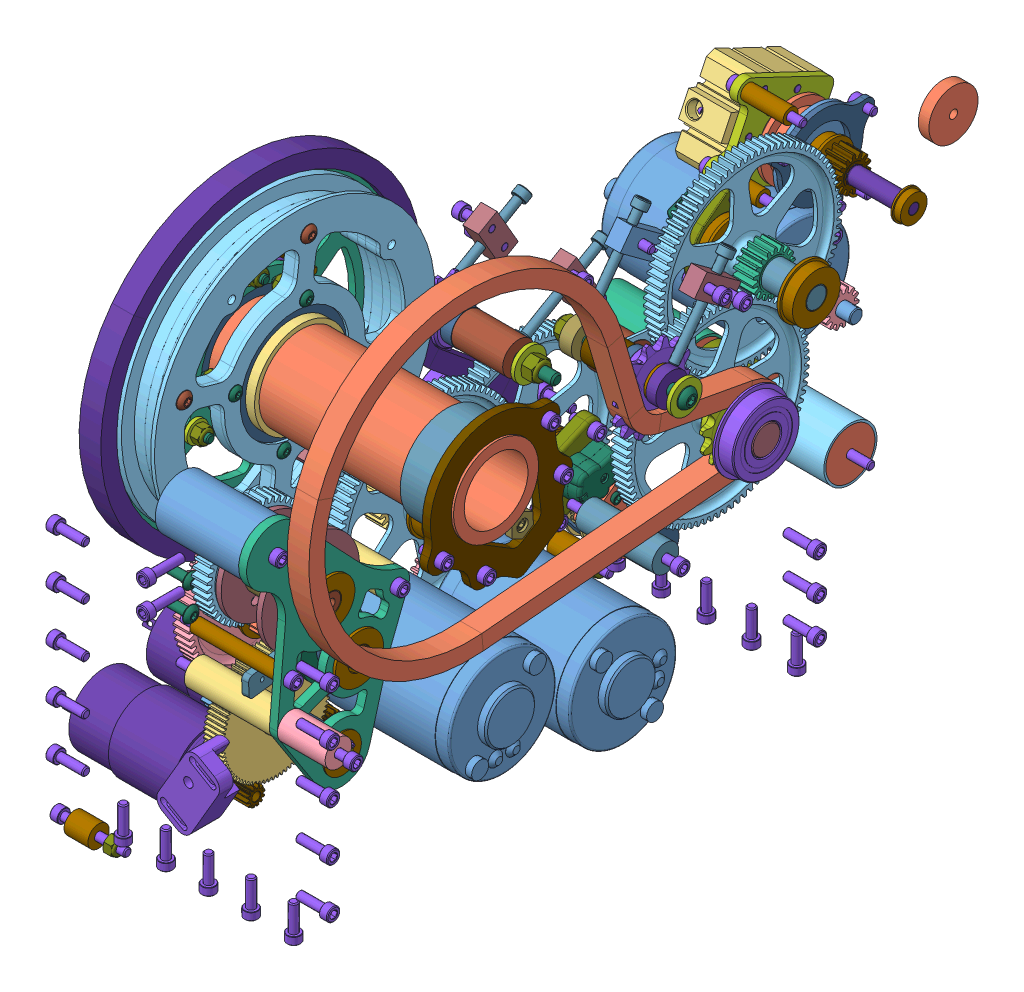
SolidWorks assembly 971-18-A-2900_Arm Gearbox, configuration Default. Lengths in mm.
Overall size (180.27 346.15 436.67).
321 component instances, 101 part files, 306 mates.
Components (placement in the parent):
- 971-18-P-0057_Arm Gearbox Plates-1: 971-18-P-0057_Arm Gearbox Plates [Not Hanger Plates] at origin size (158.75 274.35 412.07) (hidden)
- MiniCIM-1: MiniCIM [Default] at (101.9302 -45.1539 -242.57) x (-1 0 0) z (0 -0.56592 -0.82446) size (125.82 64.26 64.26)
- 971-18-P-0063_Proximal Joint Chain-1: 971-18-P-0063_Proximal Joint Chain [Default] at (142.3112 0 0) x (-1 0 0) z (0 0.942809 -0.333333) size (12.95 293.93 191.44)
- MiniCIM-2: MiniCIM [Default] at (68.2625 -128.7803 -15.3525) x (1 0 0) z (0 0.733761 -0.679407) size (125.82 64.26 64.26)
- 28T-1_2-Hex-Steel_217-5468-1: 28T-1_2-Hex-Steel_217-5468 [Default] at (42.9633 -91.1077 -64.9795) x (0 0.556138 -0.83109) z (-1 0 0) size (38.56 38.56 12.6)
- 14T-CIM_217-3414-1: 14T-CIM_217-3414 [default] at (44.9112 -128.7803 -15.3525) x (0 -0.350281 -0.936645) z (-1 0 0) size (20.32 20.6 19.05)
- 971-18-P-0186_84T Gear With Access Hole-1: 971-18-P-0186_84T Gear With Access Hole [Default] at (42.9879 -103.4997 -135.089) x (0 -0.686618 -0.727018) z (1 0 0) size (109.49 109.49 12.65)
- 971-18-P-0186_84T Gear With Access Hole-2: 971-18-P-0186_84T Gear With Access Hole [Default] at (55.5879 -91.1077 -64.9795) x (0 -0.395137 -0.918622) z (-1 0 0) size (109.49 109.49 12.65)
- 971-18-P-0186_84T Gear With Access Hole-3: 971-18-P-0186_84T Gear With Access Hole [Default] at (114.8094 -2.1568 -197.4778) x (0 0.448525 0.89377) z (-1 0 0) size (109.49 109.49 12.65)
- 971-18-P-0186_84T Gear With Access Hole-4: 971-18-P-0186_84T Gear With Access Hole [Default] at (127.4586 -58.42 -165.2367) x (0 0.119081 -0.992885) z (-1 0 0) size (109.49 109.49 12.65)
- 18T-1_2-Hex-Steel_217-5460-2: 18T-1_2-Hex-Steel_217-5460 [Default] at (127.4339 -2.1568 -197.4778) x (0 -0.996212 -0.086957) z (1 0 0) size (25.65 25.85 12.6)
- 12T_Hex_217-2662-2: 12T_Hex_217-2662 [Default] at (18.0263 -103.4997 -135.089) x (0 -0.568149 -0.822926) z (1 0 0) size (40.29 40.29 10.67)
- 6661K350_17mm ID 40mm OD BALL BEARING-2: 6661K350_17mm ID 40mm OD BALL BEARING [6661K35] at (3.53 -103.4997 -135.089) x (0 0 1) z (1 0 0) size (44.6 44.6 12)
- MiniCIM-3: MiniCIM [Default] at (68.2625 -149.225 -87.4394) x (1 0 0) z (0 0.801756 0.597652) size (125.82 64.26 64.26)
- 14T-CIM_217-3414-2: 14T-CIM_217-3414 [default] at (44.9112 -149.225 -87.4394) x (0 0.658796 0.752321) z (-1 0 0) size (20.32 20.6 19.05)
- 14T-CIM_217-3414-3: 14T-CIM_217-3414 [default] at (119.605 -45.1539 -242.57) x (0 0.994685 -0.102967) z (-1 0 0) size (20.32 20.6 19.05)
- Bearings-1: Bearings [0.5 ID, 1.125 OD, 0.313 Width, Flanged, FR8-ZZ] at (65.8876 -103.4997 -135.089) x (0 -0.204169 -0.978936) z (1 0 0) size (31.12 31.12 7.95)
- Bearings-2: Bearings [0.5 ID, 1.125 OD, 0.313 Width, Flanged, FR8-ZZ] at (3.9624 -91.1077 -64.9795) x (0 -0.438567 -0.898699) z (-1 0 0) size (31.12 31.12 7.95)
- Bearings-4: Bearings [0.5 ID, 1.125 OD, 0.313 Width, Flanged, FR8-ZZ] at (154.7876 -2.1568 -197.4778) x (0 -0.31213 0.950039) z (1 0 0) size (31.12 31.12 7.95)
- Bearings-5: Bearings [0.5 ID, 1.125 OD, 0.313 Width, Flanged, FR8-ZZ] at (104.3051 -2.1568 -197.4778) x (0 0.974827 0.222965) z (-1 0 0) size (31.12 31.12 7.95)
- Bearings-6: Bearings [0.5 ID, 1.125 OD, 0.313 Width, Flanged, FR8-ZZ] at (65.8876 -91.1077 -64.9795) x (0 0.620593 0.784133) z (1 0 0) size (31.12 31.12 7.95)
- 12T_Hex_217-2662-5: 12T_Hex_217-2662 [Default] at (142.3112 -58.42 -165.2367) x (0 -0.053723 0.998556) z (-1 0 0) size (40.29 40.29 10.67)
- 6661K350_17mm ID 40mm OD BALL BEARING-3: 6661K350_17mm ID 40mm OD BALL BEARING [6661K35] at (155.22 -58.42 -165.2367) x (0 -0.924225 -0.381849) z (-1 0 0) size (44.6 44.6 12)
- 3549S-1BA-102B-ND 10 turn potentiometer-1: 3549S-1BA-102B-ND 10 turn potentiometer [Default] at (93.141 -149.8585 -169.7731) x (0 -0.445388 -0.895338) z (-1 0 0) size (22.48 22.48 39.06)
- 3547S-1AA-102A-ND 3 Turn Potentiometer Bourns-2: 3547S-1AA-102A-ND 3 Turn Potentiometer Bourns [Default] at (64.1081 -58.42 -165.2367) x (0 0.520541 -0.853837) z (1 0 0) size (22.48 22.48 39.06)
- Bearings-9: Bearings [0.5 ID, 1.125 OD, 0.313 Width, Flanged, FR8-ZZ] at (104.3051 -58.42 -165.2367) x (0 -0.997236 -0.074294) z (-1 0 0) size (31.12 31.12 7.95)
- SHCS-1: SHCS [6.5, #10-32] at (82.55 45.4322 -285.7008) x (1 0 0) z (0 -0.658646 -0.752453) size (170.15 7.92 7.92) (hidden)
- SRK Mag Encoder Magnet-1: SRK Mag Encoder Magnet [Default] at (63.0047 -103.4997 -135.089) x (0 0.994372 0.105943) z (0 0.105943 -0.994372) size (6.35 12.7 6.35)
- SRK Mag Encoder Magnet-2: SRK Mag Encoder Magnet [Default] at (107.2515 -2.1568 -197.4778) x (0 -0.949695 0.313176) z (0 -0.313176 -0.949695) size (6.35 12.7 6.35)
- 971-18-P-0104_Arm Gearbox Proximal Arm Output Shaft-1: 971-18-P-0104_Arm Gearbox Proximal Arm Output Shaft [Default] at (161.22 -58.42 -165.2367) x (0 0.817505 0.575921) z (1 0 0) size (19.05 19.05 69.68)
- 971-18-P-0105_Arm Gearbox Proximal Arm First Stage Shaft -1: 971-18-P-0105_Arm Gearbox Proximal Arm First Stage Shaft  [Default] at (133.7437 -2.1568 -197.4778) x (0 0 -1) z (1 0 0) size (15.88 15.88 58.37)
- 971-18-P-0106_Arm Gearbox Distal Arm First Stage Shaft-1: 971-18-P-0106_Arm Gearbox Distal Arm First Stage Shaft [Default] at (69.8627 -91.1077 -64.9795) x (0 0 -1) z (1 0 0) size (15.88 15.88 69.88)
- 971-18-P-0107_Arm Gearbox Distal Arm Output Shaft-1: 971-18-P-0107_Arm Gearbox Distal Arm Output Shaft [Default] at (69.8627 -103.4997 -135.089) x (0 0.391562 -0.920152) z (1 0 0) size (19.05 19.05 72.33)
- 971-18-P-0070_Distal Joint Chain-1: 971-18-P-0070_Distal Joint Chain [Default] at (18.0263 0 0) x (-1 0 0) z (0 0.793801 -0.608178) size (12.95 288.85 191.44)
- 971-18-P-0101_Tensioner Strap-1: 971-18-P-0101_Tensioner Strap [Default] x (-1 0 0) z (0 0.537919 -0.842996) size (4.76 92.32 90.96)
- 971-18-P-0101_Tensioner Strap-2: 971-18-P-0101_Tensioner Strap [Default] at (163.5125 0 0) x (-1 0 0) z (0 0.537919 -0.842996) size (4.76 92.32 90.96)
- potentiometer belt-1: potentiometer belt [Default] at (51.6937 -103.4997 -135.089) x (1 0 0) z (0 0.800703 0.599061) size (6.35 27.13 83.74)
- 971-18-P-0112_Arm Gearbox Distal Potentiometer Mount-1: 971-18-P-0112_Arm Gearbox Distal Potentiometer Mount [Default] at (74.695 -149.8585 -169.7731) x (-1 0 0) z (0 0.599061 -0.800703) size (8.89 42.86 25.08)
- A-6z16-036df2508_36t plastic pulley-1: A-6z16-036df2508_36t plastic pulley [Default] at (54.8687 -149.8585 -169.7731) x (0 -0.600937 0.799296) z (1 0 0) size (27.69 27.69 17.46)
- 971-18-P-0254_40T plastic pulley hex-1: 971-18-P-0254_40T plastic pulley hex [Default] at (54.8687 -103.4997 -135.089) x (0 -0.910247 0.414066) z (-1 0 0) size (30.23 30.23 11.11)
- 971-18-P-0116_Arm Proximal Side Spacer-1: 971-18-P-0116_Arm Proximal Side Spacer [Default] at (129.54 -99.4146 -224.1283) x (1 0 0) z (0 -0.998204 -0.059903) size (45.72 31.75 31.75)
- 971-18-P-0116_Arm Proximal Side Spacer-2: 971-18-P-0116_Arm Proximal Side Spacer [Default] at (129.54 45.4322 -285.7008) x (1 0 0) z (0 -0.135571 0.990768) size (45.72 31.75 31.75) (hidden)
- 971-18-P-0115_Arm Distal Side Spacer-1: 971-18-P-0115_Arm Distal Side Spacer [Default] at (34.925 -99.4146 -224.1283) x (1 0 0) z (0 -0.874507 -0.485014) size (57.15 31.75 31.75)
- 971-18-P-0115_Arm Distal Side Spacer-2: 971-18-P-0115_Arm Distal Side Spacer [Default] at (34.925 -166.289 -43.6572) x (1 0 0) z (0 0.434751 -0.900551) size (57.15 31.75 31.75)
- 971-18-P-0118_Arm Distal Side Double Spacer-1: 971-18-P-0118_Arm Distal Side Double Spacer [Default] at (54.1401 45.4322 -285.7008) x (1 0 0) z (0 -0.790861 -0.611996) size (95.58 31.75 31.75) (hidden)
- 971-18-A-4500_Arm Tensioner Idler-1: 971-18-A-4500_Arm Tensioner Idler [Default] at (136.9581 -12.6592 -117.4327) x (0 0.639462 0.768823) z (-1 0 0) size (46.24 46.24 19.05)
  - 8491A293_0_5 OD PRESS-FIT DRILL BUSHING-1: 8491A293_0_5 OD PRESS-FIT DRILL BUSHING [8491A293] at origin size (12.7 12.7 19.05)
  - 971-18-P-0119_Arm Tensioner Idler-1: 971-18-P-0119_Arm Tensioner Idler [Default] at (0 0 -5.353) x (0.987019 -0.160606 0) z (0 0 1) size (40.29 40.29 10.67)
  - 5905K230_0_5ID STEEL NEEDLE-ROLLER BEARING-1: 5905K230_0_5ID STEEL NEEDLE-ROLLER BEARING [5905K23] at (0 0 -3.175) size (17.46 17.46 12.7)
  - VexPro_Hex Spacers-2: VexPro_Hex Spacers [1_2 Hex, 0.25] at (0 0 6.35) x (0.957977 0.286844 0) z (0 0 1) size (19.51 19.51 6.35)
- 971-18-A-4500_Arm Tensioner Idler-2: 971-18-A-4500_Arm Tensioner Idler [Default] at (23.3793 -39.637 -114.8895) x (0 -0.847075 -0.531473) z (1 0 0) size (46.24 46.24 19.05)
  - 8491A293_0_5 OD PRESS-FIT DRILL BUSHING-1: 8491A293_0_5 OD PRESS-FIT DRILL BUSHING [8491A293] at origin size (12.7 12.7 19.05)
  - 971-18-P-0119_Arm Tensioner Idler-1: 971-18-P-0119_Arm Tensioner Idler [Default] at (0 0 -5.353) x (0.987019 -0.160606 0) z (0 0 1) size (40.29 40.29 10.67)
  - 5905K230_0_5ID STEEL NEEDLE-ROLLER BEARING-1: 5905K230_0_5ID STEEL NEEDLE-ROLLER BEARING [5905K23] at (0 0 -3.175) size (17.46 17.46 12.7)
  - VexPro_Hex Spacers-2: VexPro_Hex Spacers [1_2 Hex, 0.25] at (0 0 6.35) x (0.957977 0.286844 0) z (0 0 1) size (19.51 19.51 6.35)
- 971-18-P-0122_Distal Tensioner Long Spacer-1: 971-18-P-0122_Distal Tensioner Long Spacer [Default] at (48.1951 -39.637 -114.8895) x (0 0 1) z (-1 0 0) size (19.05 19.05 30.58)
- 971-18-P-0123_Distal Tensioner Short Spacer-1: 971-18-P-0123_Distal Tensioner Short Spacer [Default] at (10.1078 -39.637 -114.8895) x (0 0.086251 0.996273) z (-1 0 0) size (19.05 19.05 7.49)
- 971-18-P-0124_Sketchy Chain Tensioner-1: 971-18-P-0124_Sketchy Chain Tensioner [Default] at (11.1125 -19.1237 -150.4225) x (1 0 0) z (0 0.866025 0.5) size (9.53 12.7 25.4)
- 90044A120_2-in Full Thread BLACK-OXIDE ALLOY STEEL SOCKET HEAD CAP SCREW-1: 90044A120_2-in Full Thread BLACK-OXIDE ALLOY STEEL SOCKET HEAD CAP SCREW [90044A120] at (11.1125 -22.1758 -145.1362) x (0 -0.5 0.866025) z (-0.011915 0.865964 0.499965) size (55.85 7.92 7.92)
- 971-18-P-0124_Sketchy Chain Tensioner-2: 971-18-P-0124_Sketchy Chain Tensioner [Default] at (58.7375 -19.1237 -150.4225) x (1 0 0) z (0 0.866025 0.5) size (9.53 12.7 25.4)
- 90044A120_2-in Full Thread BLACK-OXIDE ALLOY STEEL SOCKET HEAD CAP SCREW-2: 90044A120_2-in Full Thread BLACK-OXIDE ALLOY STEEL SOCKET HEAD CAP SCREW [90044A120] at (58.7375 -22.1758 -145.1362) x (0 -0.5 0.866025) z (-0.011915 0.865964 0.499965) size (55.85 7.92 7.92)
- BHCS-1: BHCS [3.5, .25-20] at (-5.6388 -39.637 -114.8895) x (0 0 1) z (-1 0 0) size (11.1 11.1 92.48)
- Nylon-Insert Locknut-1: Nylon-Insert Locknut [.25-20  Nylon-Insert Locknut] at (70.5485 -39.637 -114.8895) x (0 -0.87684 0.480783) z (0 0.480783 0.87684) size (11.11 7.94 12.83)
- 971-18-P-0248_Proximal Tensioner Short Spacer-2: 971-18-P-0248_Proximal Tensioner Short Spacer [Default] at (149.4359 -12.6592 -117.4327) x (0 -0.700571 0.713583) z (-1 0 0) size (19.05 19.05 5.91)
- 971-18-P-0124_Sketchy Chain Tensioner-3: 971-18-P-0124_Sketchy Chain Tensioner [Default] at (147.6375 24.7667 -144.9822) x (1 0 0) z (0 0.592784 0.805361) size (9.53 12.7 25.4)
- 90044A120_2-in Full Thread BLACK-OXIDE ALLOY STEEL SOCKET HEAD CAP SCREW-3: 90044A120_2-in Full Thread BLACK-OXIDE ALLOY STEEL SOCKET HEAD CAP SCREW [90044A120] at (147.6375 15.467 -138.1372) x (0 -0.805361 0.592784) z (-0.011915 0.592742 0.805304) size (55.85 7.92 7.92)
- 971-18-P-0125_Proximal Tensioner Long Spacer-1: 971-18-P-0125_Proximal Tensioner Long Spacer [Default] at (117.07 -12.6592 -117.4327) x (0 0 -1) z (1 0 0) size (17.78 17.78 20.73)
- 90044A120_2-in Full Thread BLACK-OXIDE ALLOY STEEL SOCKET HEAD CAP SCREW-4: 90044A120_2-in Full Thread BLACK-OXIDE ALLOY STEEL SOCKET HEAD CAP SCREW [90044A120] at (97.1677 14.9556 -137.7608) x (0 -0.805361 0.592784) z (0.19068 0.581908 0.790585) size (55.85 7.92 7.92)
- BHCS-2: BHCS [3, .25-20] at (164.3888 -12.6592 -117.4327) x (0 -0.924225 -0.381849) z (1 0 0) size (11.1 11.1 79.78)
- Nylon-Insert Locknut-2: Nylon-Insert Locknut [.25-20  Nylon-Insert Locknut] at (94.4372 -12.6592 -117.4327) x (0 -0.381849 0.924225) z (0 -0.924225 -0.381849) size (11.11 7.94 12.83)
- 971-18-P-0123_Distal Tensioner Short Spacer-3: 971-18-P-0123_Distal Tensioner Short Spacer [Default] at (98.1837 -12.6592 -117.4327) x (0 -0.700571 0.713583) z (-1 0 0) size (19.05 19.05 7.49)
- 971-18-P-0264_Swoopy thing 2-1: 971-18-P-0264_Swoopy thing 2 [Default] at (97.1677 24.7667 -144.9822) x (1 0 0) z (0 -0.592784 -0.805361) size (9.53 12.7 29.21)
- 971-18-P-0119_Arm Tensioner Idler-1: 971-18-P-0119_Arm Tensioner Idler [Default] at (142.3112 -18.7027 -112.9867) x (0 0.507683 0.861544) z (-1 0 0) size (40.29 40.29 10.67)
- 971-18-A-4800_Arm Base Axle-1: 971-18-A-4800_Arm Base Axle [Default] at (79.375 0 0) x (0 0.839057 0.544043) z (1 0 0) size (228.13 188.75 173.98)
  - 971-18-P-0098_Proximal Shoulder Joint Tube Shaft-1: 971-18-P-0098_Proximal Shoulder Joint Tube Shaft [Default] at origin size (50.8 50.8 173.98)
  - 971-18-P-0109_Arm to Capstan Spacer-1: 971-18-P-0109_Arm to Capstan Spacer [Default] at (0 0 -33.6475) size (55.56 55.56 5.38)
  - 971-18-P-0110_Capstan to Gearbox Spacer-1: 971-18-P-0110_Capstan to Gearbox Spacer [Default] at (0 0 -70.6322) x (0.975154 0.22153 0) z (0 0 1) size (55.56 55.56 4.72)
  - 971-18-A-2700_Distal Joint Base Sprocket-1: 971-18-A-2700_Distal Joint Base Sprocket [Default] at (0 0 -45.7212) x (0 0 -1) z (-0.006536 0.999979 0) size (39.06 226.91 187.27)
    - 971-18-P-0065_Distal Joint Capstan-1: 971-18-P-0065_Distal Joint Capstan [Default] at origin size (24.51 167.64 167.64)
    - 971-18-P-0069_Distal Base Sprocket, 60T #35-1: 971-18-P-0069_Distal Base Sprocket, 60T #35 [Default] at (15.64 0 0) x (0 0 1) z (-1 0 0) size (187.27 187.27 4.29)
    - Mock Allen Key-1: Mock Allen Key [Default] at (0 33.0633 -17.145) x (0.575263 0.315216 -0.754792) z (0.20677 -0.948834 -0.238663) size (4.57 4.57 127) (hidden)
    - 91525A318_No8 Oversized Washer-1: 91525A318_No8 Oversized Washer [91525A318] at (-2.3813 -26.2838 -25.4) x (1 0 0) z (0 0.858193 0.513327) size (2.03 12.7 12.7)
    - Nylon-Insert Locknut-1: Nylon-Insert Locknut [#8-32  Nylon-Insert Locknut] at (-0.3493 -26.2838 -25.4) x (0 -0.163443 -0.986553) z (0 -0.986553 0.163443) size (8.73 5.95 10.08)
    - 971-18-P-0067_Distal Sprocket Bearing Reinforcement-1: 971-18-P-0067_Distal Sprocket Bearing Reinforcement [Default] at (17.7863 0 0) x (1 0 0) z (0 0.5 0.866025) size (4.76 97.7 86.31)
    - BHCS-4: BHCS [0.75, #10-32] at (25.1143 -36.8061 -21.25) x (0 -0.437304 -0.899314) z (1 0 0) size (9.17 9.17 21.8)
    - Dowel Pins-1: Dowel Pins [0.1875" OD, 0.375" Length] at (17.7863 -36.8061 21.25) x (1 0 0) z (0 0.150684 0.988582) size (9.53 4.76 4.76)
    - Dowel Pins-2: Dowel Pins [0.1875" OD, 0.375" Length] at (17.7863 36.8061 21.25) x (1 0 0) z (0 0.780795 -0.624787) size (9.53 4.76 4.76)
    - Dowel Pins-3: Dowel Pins [0.1875" OD, 0.375" Length] at (17.7863 0 -42.5) x (1 0 0) z (0 -0.931479 -0.363795) size (9.53 4.76 4.76)
    - BHCS-7: BHCS [0.75, #10-32] at (25.1143 0 42.5) x (0 -0.560177 0.828373) z (1 0 0) size (9.17 9.17 21.8)
    - BHCS-8: BHCS [0.75, #10-32] at (25.1143 36.8061 -21.25) x (0 0.997481 0.070941) z (1 0 0) size (9.17 9.17 21.8)
    - 50mm x 65mm x 7mm-2: 50mm x 65mm x 7mm [Default] at (15.5488 0 0) x (1 0 0) z (0 0.999973 -0.007282) size (7 65 65)
    - 50mm x 65mm x 7mm-3: 50mm x 65mm x 7mm [Default] at (-9.3813 0 0) x (1 0 0) z (0 0.591037 0.806644) size (7 65 65)
    - 91525A318_No8 Oversized Washer-6: 91525A318_No8 Oversized Washer [91525A318] at (-0.3493 26.2838 -25.4) x (-1 0 0) z (0 -0.146729 -0.989177) size (2.03 12.7 12.7)
    - 91525A318_No8 Oversized Washer-7: 91525A318_No8 Oversized Washer [91525A318] at (-2.3813 -26.2838 25.4) x (1 0 0) z (0 0.982147 0.188113) size (2.03 12.7 12.7)
    - 91525A318_No8 Oversized Washer-8: 91525A318_No8 Oversized Washer [91525A318] at (-0.3493 26.2838 25.4) x (-1 0 0) z (0 -0.146729 -0.989177) size (2.03 12.7 12.7)
    - Dowel Pins-4: Dowel Pins [0.1875" OD, 1" Length] at (5.0863 0 -69.215) size (25.4 4.76 4.76)
    - Dowel Pins-5: Dowel Pins [0.1875" OD, 1" Length] at (5.0863 0 69.215) x (1 0 0) z (0 -0.930216 0.367012) size (25.4 4.76 4.76)
    - Dowel Pins-8: Dowel Pins [0.1875" OD, 1" Length] at (5.0863 -68.58 0) x (1 0 0) z (0 -0.930216 0.367012) size (25.4 4.76 4.76)
    - Nylon-Insert Locknut-6: Nylon-Insert Locknut [#8-32  Nylon-Insert Locknut] at (-0.3493 26.2838 -25.4) x (0 0.24471 -0.969596) z (0 -0.969596 -0.24471) size (8.73 5.95 10.08)
    - Nylon-Insert Locknut-7: Nylon-Insert Locknut [#8-32  Nylon-Insert Locknut] at (-0.3493 26.2838 25.4) x (0 -0.163443 -0.986553) z (0 -0.986553 0.163443) size (8.73 5.95 10.08)
    - Nylon-Insert Locknut-8: Nylon-Insert Locknut [#8-32  Nylon-Insert Locknut] at (-0.3493 -26.2838 25.4) x (0 -0.619554 0.784954) z (0 0.784954 0.619554) size (8.73 5.95 10.08)
    - BHCS-14: BHCS [0.75, #8-32] at (-13.2271 -26.2838 -25.4) x (0 0.924225 0.381849) z (-1 0 0) size (7.92 7.92 21.4)
    - BHCS-15: BHCS [0.75, #8-32] at (-13.2271 26.2838 -25.4) x (0 0.924225 0.381849) z (-1 0 0) size (7.92 7.92 21.4)
    - BHCS-16: BHCS [0.75, #8-32] at (-13.2271 26.2838 25.4) x (0 0.924225 0.381849) z (-1 0 0) size (7.92 7.92 21.4)
    - BHCS-17: BHCS [0.75, #8-32] at (-13.2271 -26.2838 25.4) x (0 0.924225 0.381849) z (-1 0 0) size (7.92 7.92 21.4)
    - 91525A318_No8 Oversized Washer-9: 91525A318_No8 Oversized Washer [91525A318] at (13.4938 36.8061 -21.25) x (-1 0 0) z (0 -0.146729 -0.989177) size (2.03 12.7 12.7)
    - Nylon-Insert Locknut-9: Nylon-Insert Locknut [#8-32  Nylon-Insert Locknut] at (11.4618 -36.8061 -21.25) x (0 -0.947533 0.319658) z (0 -0.319658 -0.947533) size (8.73 5.95 10.08)
    - 91525A318_No8 Oversized Washer-10: 91525A318_No8 Oversized Washer [91525A318] at (13.4938 -36.8061 -21.25) x (-1 0 0) z (0 -0.146729 -0.989177) size (2.03 12.7 12.7)
    - 91525A318_No8 Oversized Washer-11: 91525A318_No8 Oversized Washer [91525A318] at (11.4618 0 42.5) x (1 0 0) z (0 0.858193 0.513327) size (2.03 12.7 12.7)
    - Nylon-Insert Locknut-10: Nylon-Insert Locknut [#8-32  Nylon-Insert Locknut] at (11.4618 0 42.5) x (0 -0.947533 0.319658) z (0 -0.319658 -0.947533) size (8.73 5.95 10.08)
    - Nylon-Insert Locknut-11: Nylon-Insert Locknut [#8-32  Nylon-Insert Locknut] at (11.4618 36.8061 -21.25) x (0 -0.947533 0.319658) z (0 -0.319658 -0.947533) size (8.73 5.95 10.08)
    - Nylon-Insert Locknut-12: Nylon-Insert Locknut [#8-32  Nylon-Insert Locknut] at (17.7863 -53.0218 44.4905) x (0 -0.163443 -0.986553) z (0 -0.986553 0.163443) size (8.73 5.95 10.08)
    - Nylon-Insert Locknut-13: Nylon-Insert Locknut [#8-32  Nylon-Insert Locknut] at (17.7863 -53.0218 -44.4905) x (0 -0.163443 -0.986553) z (0 -0.986553 0.163443) size (8.73 5.95 10.08)
    - Nylon-Insert Locknut-14: Nylon-Insert Locknut [#8-32  Nylon-Insert Locknut] at (17.7863 53.0218 -44.4905) x (0 -0.163443 -0.986553) z (0 -0.986553 0.163443) size (8.73 5.95 10.08)
    - Nylon-Insert Locknut-15: Nylon-Insert Locknut [#8-32  Nylon-Insert Locknut] at (17.7863 53.0218 44.4905) x (0 -0.163443 -0.986553) z (0 -0.986553 0.163443) size (8.73 5.95 10.08)
    - Dowel Pins-10: Dowel Pins [0.1875" OD, 1" Length] at (5.0863 68.58 -19.05) size (25.4 4.76 4.76)
    - Dowel Pins-11: Dowel Pins [0.1875" OD, 1" Length] at (5.0863 68.58 19.05) size (25.4 4.76 4.76)
    - 92949A827_18-8 SS 10-32 1_375 BHCS-1: 92949A827_18-8 SS 10-32 1_375 BHCS [92949A827] at (-13.5826 -53.0218 44.4905) x (0 0 1) z (-1 0 0) size (9.17 9.17 37.67)
    - 92949A827_18-8 SS 10-32 1_375 BHCS-2: 92949A827_18-8 SS 10-32 1_375 BHCS [92949A827] at (-13.5826 53.0218 44.4905) x (0 0 1) z (-1 0 0) size (9.17 9.17 37.67)
    - 92949A827_18-8 SS 10-32 1_375 BHCS-3: 92949A827_18-8 SS 10-32 1_375 BHCS [92949A827] at (-13.5826 -53.0218 -44.4905) x (0 0 1) z (-1 0 0) size (9.17 9.17 37.67)
    - 92949A827_18-8 SS 10-32 1_375 BHCS-4: 92949A827_18-8 SS 10-32 1_375 BHCS [92949A827] at (-13.5826 53.0218 -44.4905) x (0 0 1) z (-1 0 0) size (9.17 9.17 37.67)
    - 3-16 in wire rope stop-2: 3-16 in wire rope stop [Default] at (0 50.8751 5.4991) size (10.72 7.94 10.72)
    - 971-18-P-0259_Distal Joint Crimp Block-1: 971-18-P-0259_Distal Joint Crimp Block [Default] at (0 59.6063 0) x (0 -1 0) z (0 0 1) size (4.76 14.1 38.1)
    - 3-16 in wire rope stop-3: 3-16 in wire rope stop [Default] at (0 50.8751 -5.4991) size (10.72 7.94 10.72)
  - 971-18-P-0111_Arm to Gearbox Spacer-1: 971-18-P-0111_Arm to Gearbox Spacer [Default] at (0 0 64.5171) size (55.56 55.56 16.95)
  - 98541A167_50 mm BLACK-FINISH STEEL EXTERNAL RETAINING RING-1: 98541A167_50 mm BLACK-FINISH STEEL EXTERNAL RETAINING RING [98541A167] at (0 0 -85.2645) x (0 0 -1) z (1 0 0) size (2 57.8 54.19)
- 971-18-P-0130_Arm Middle Spacer-1: 971-18-P-0130_Arm Middle Spacer [Default] at (85.09 -99.4146 -224.1283) x (1 0 0) z (0 0.062055 0.998073) size (33.68 31.75 31.75)
- Bearings-10: Bearings [10.25mm ID, 0.875 OD, 0.281 Width, Flanged, ThunderHex] at (104.7115 12.3866 -258.0628) x (0 -0.869205 0.494452) z (-1 0 0) size (24.61 24.61 7.14)
- Bearings-11: Bearings [0.25 ID, 0.625 OD, 0.196 Width, Flanged, FR4-2Z] at (153.8732 12.3866 -258.0628) x (0 0.663133 0.748502) z (1 0 0) size (17.53 17.53 4.98)
- 971-18-P-0143_Arm Brake Shaft-1: 971-18-P-0143_Arm Brake Shaft [Default] at (120.9802 12.3866 -258.0628) x (0 0.04476 0.998998) z (1 0 0) size (11 9.53 69.09)
- 14T-3_8-Hex-Steel_217-3100-1: 14T-3_8-Hex-Steel_217-3100 [default] at (114.6302 12.3866 -258.0628) x (0 0 1) z (-1 0 0) size (20.32 20.6 12.7)
- 971-18-A-4900_Brake Assembly-1: 971-18-A-4900_Brake Assembly [Default] at (71.628 12.3866 -258.0628) x (-1 0 0) z (0 0.902882 -0.429889) size (63.63 72.45 63.23)
  - 971-18-P-0146_Brake Disc-1: 971-18-P-0146_Brake Disc [Default] at (-27.1272 0 0) x (0 -0.921218 0.389046) z (1 0 0) size (48.26 48.26 13.21)
  - Bearings-1: Bearings [0.5 ID, 1.125 OD, 0.313 Width, R8-ZZ] at (-20.1041 0 0) x (0 0.976049 -0.217552) z (1 0 0) size (28.57 28.57 7.95)
  - 971-18-P-0149_Brake Disc Pusher-1: 971-18-P-0149_Brake Disc Pusher [Default] at (-22.4917 0 0) x (0 -0.872177 -0.48919) z (-1 0 0) size (38.1 38.1 17.28)
  - NCQ8B150-012S-1: NCQ8B150-012S [Brake Config] at origin size (30.73 55.63 50.8)
    - NCQ8B150-012S_BODY-1: NCQ8B150-012S_BODY [Default] at origin size (25.53 55.63 50.8)
    - NCQ8150-012S_ROD-1: NCQ8150-012S_ROD [Default] at (-1.905 0 0) size (20.45 38.1 38.1)
  - 91255A641_3-8 1_2L ALLOY STEEL BHCS-1: 91255A641_3-8 1_2L ALLOY STEEL BHCS [91255A641] at (-13.843 0 0) x (0 0 1) z (-1 0 0) size (16.66 16.66 18.07)
  - 1561T260_STACKED WAVE DISC COMPRESSION SPRING-1: 1561T260_STACKED WAVE DISC COMPRESSION SPRING [Default] at (-26.3652 0 0) x (0 -0.99093 -0.134379) z (0 0.134379 -0.99093) size (15.24 6.1 15.24)
  - 971-18-P-0165_Brake Piston Mount-1: 971-18-P-0165_Brake Piston Mount [Default] at (-4.7625 0 0) x (1 0 0) z (0 -1 0) size (4.76 50.8 72.45)
  - SHCS-1: SHCS [1, #10-32] at (7.747 19.685 19.685) x (-1 0 0) z (0 -0.045421 -0.998968) size (30.45 7.92 7.92)
  - SHCS-2: SHCS [1, #10-32] at (7.747 -2.2352 19.685) x (-1 0 0) z (0 -0.045421 -0.998968) size (30.45 7.92 7.92)
  - SHCS-3: SHCS [1, #10-32] at (7.747 19.685 -2.2352) x (-1 0 0) z (0 -0.045421 -0.998968) size (30.45 7.92 7.92)
  - SHCS-4: SHCS [1, #10-32] at (7.747 -2.2352 -2.2352) x (-1 0 0) z (0 -0.045421 -0.998968) size (30.45 7.92 7.92)
  - No 10 Aluminum Spacer-1: No 10 Aluminum Spacer [0.5" OD, 1" Length] at (-17.4625 30.1625 19.05) x (0 0 1) z (-1 0 0) size (8.89 8.89 25.4)
  - SHCS-5: SHCS [1.5, #10-32] at (-19.05 30.1625 19.05) x (-1 0 0) z (0 0.859608 -0.510953) size (43.15 7.92 7.92)
  - No 10 Aluminum Spacer-2: No 10 Aluminum Spacer [0.5" OD, 1" Length] at (-17.4625 30.1625 -19.05) x (0 0 1) z (-1 0 0) size (8.89 8.89 25.4)
  - No 10 Aluminum Spacer-3: No 10 Aluminum Spacer [0.5" OD, 1" Length] at (-17.4625 -29.591 -15.24) x (0 0 1) z (-1 0 0) size (8.89 8.89 25.4)
  - SHCS-6: SHCS [1.5, #10-32] at (-19.05 30.1625 -19.05) x (-1 0 0) z (0 0.859608 -0.510953) size (43.15 7.92 7.92)
  - SHCS-7: SHCS [1.5, #10-32] at (-19.05 -29.591 -15.24) x (-1 0 0) z (0 0.859608 -0.510953) size (43.15 7.92 7.92)
- 971-18-P-0148_Brake Pad-1: 971-18-P-0148_Brake Pad [Default] at (98.7552 12.3866 -258.0628) x (1 0 0) z (0 0.909675 0.41532) size (3.17 57.78 60.11)
- 599-23-Prometheus-ARM-P-4025-1: 599-23-Prometheus-ARM-P-4025 [Default] at (101.1428 12.3866 -258.0628) x (0 0.835687 -0.549206) z (1 0 0) size (15.88 15.88 1.02)
- 84865A130_10-32 Mitebite LOW-PROFILE CLAMP-1: 84865A130_10-32 Mitebite LOW-PROFILE CLAMP [84865A13] at (-3.5814 -27.627 -17.6289) x (0 -0.537919 0.842996) z (-1 0 0) size (14.66 12.7 12.96)
- 84865A130_10-32 Mitebite LOW-PROFILE CLAMP-2: 84865A130_10-32 Mitebite LOW-PROFILE CLAMP [84865A13] at (162.3314 -27.627 -17.6289) x (0 0.537919 -0.842996) z (1 0 0) size (14.66 12.7 12.96)
- 1_2in Shaft Collar, 217-2736-1: 1_2in Shaft Collar, 217-2736 [default] at (98.6093 -60.1845 -160.3259) x (0 0.179121 0.983827) z (-1 0 0) size (25.39 25.4 6.35)
- SHCS-2: SHCS [0.3125, #10-32] at (102.7239 24.3862 -284.3456) x (1 0 0) z (0 -0.100604 0.994927) size (12.99 7.92 7.92)
- SHCS-3: SHCS [0.3125, #10-32] at (102.7239 24.8072 -231.9763) x (1 0 0) z (0 -0.697491 -0.716594) size (12.99 7.92 7.92)
- SHCS-4: SHCS [0.3125, #10-32] at (102.7239 -15.5806 -265.3162) x (1 0 0) z (0 0.997281 -0.073692) size (12.99 7.92 7.92)
- SHCS-5: SHCS [0.5, #10-32] at (100.3427 -24.2127 -256.9444) x (-1 0 0) z (0 -0.957951 -0.286931) size (17.75 7.92 7.92)
- SHCS-6: SHCS [0.5, #10-32] at (100.3427 -66.0952 -228.1956) x (-1 0 0) z (0 -0.957951 -0.286931) size (17.75 7.92 7.92)
- SHCS-7: SHCS [0.5, #10-32] at (69.85 -111.5234 3.285) x (1 0 0) z (0 0.100604 -0.994927) size (17.75 7.92 7.92)
- SHCS-8: SHCS [0.5, #10-32] at (69.85 -164.4054 -67.0748) x (1 0 0) z (0 0.100604 -0.994927) size (17.75 7.92 7.92)
- SHCS-9: SHCS [0.5, #10-32] at (69.85 -134.0446 -107.804) x (1 0 0) z (0 0.100604 -0.994927) size (17.75 7.92 7.92)
- SHCS-10: SHCS [0.5, #10-32] at (69.85 -146.0373 -33.9901) x (1 0 0) z (0 0.100604 -0.994927) size (17.75 7.92 7.92)
- 971-18-A-6600_Arm Hard Stop-1: 971-18-A-6600_Arm Hard Stop [Default] at (322.2008 44.3878 -77.0031) x (0 0.866025 0.5) z (1 0 0) size (98.86 50.8 71.5) (hidden)
  - 971-18-P-0133_Arm hard stop-1: 971-18-P-0133_Arm hard stop [Default] at (-76.7744 -181.2597 -202.8081) size (98.86 50.8 71.5) (hidden)
  - BHCS-1: BHCS [1, #10-32] at (-71.6944 -196.5251 -202.8081) x (-0.557244 0 -0.830349) z (0 -1 0) size (9.17 9.17 28.15)
  - Nylon-Insert Locknut-1: Nylon-Insert Locknut [#10-32  Nylon-Insert Locknut] at (-71.6944 -176.5607 -202.8081) x (0.866025 0 -0.5) z (0.5 0 0.866025) size (9.53 5.95 11)
- 971-18-P-0185_Arm cross small standoff-1: 971-18-P-0185_Arm cross small standoff [Default] at (129.54 -98.1413 -113.6751) x (0 0 1) z (-1 0 0) size (15.88 15.88 45.69)
- 971-18-A-5400_SRX Mag Encoder 15 Assembly-1: 971-18-A-5400_SRX Mag Encoder 15 Assembly [Default] at (93.9927 -2.1568 -197.4778) x (1 0 0) z (0 0.939693 -0.34202) size (26.21 36.17 52.86)
  - SRX Mag Encoder 15-697867-1: SRX Mag Encoder 15-697867 [Default] at (21.59 0 0) x (0 0.766044 0.642788) z (-1 0 0) size (21.75 26.91 13.62)
  - 971-18-P-0205_SRX Mag Encoder 15 Mount-3: 971-18-P-0205_SRX Mag Encoder 15 Mount [Default] at origin size (7.94 34.29 52.86)
  - SHCS-1: SHCS [0.5, #10-32] at (6.35 0 -20.955) x (1 0 0) z (0 -0.100604 0.994927) size (17.75 7.92 7.92)
  - SHCS-2: SHCS [0.5, #10-32] at (6.35 0 20.955) x (1 0 0) z (0 -0.100604 0.994927) size (17.75 7.92 7.92)
- 971-18-A-5700_Winch Gearbox-1: 971-18-A-5700_Winch Gearbox [Default] at origin size (175.5 205.56 123.38)
  - 217-4347 775pro-1: 217-4347 775pro [Default] at (63.5 -164.211 65.8368) x (-1 0 0) z (0 -0.917648 0.397394) size (88 44.6 44.6)
  - 217-4347 775pro-2: 217-4347 775pro [Default] at (63.5 -148.8359 19.5559) x (-1 0 0) z (0 -0.810988 0.585062) size (88 44.6 44.6)
  - Bearings-1: Bearings [10.25mm ID, 0.875 OD, 0.281 Width, Flanged, ThunderHex] at (66.2813 -130.6355 51.2967) x (0 0.937169 0.348877) z (-1 0 0) size (24.61 24.61 7.14)
  - Bearings-2: Bearings [13.75mm ID, 1.125 OD, 0.313 Width, Flanged, ThunderHex] at (65.8749 -85.7748 42.0871) x (0 0.860152 0.510038) z (-1 0 0) size (31.12 31.12 7.95)
  - Bearings-3: Bearings [0.5 ID, 1.125 OD, 0.313 Width, Flanged, FR8-ZZ] at (65.8749 -48.786 59.1058) x (0 0.900252 0.43537) z (-1 0 0) size (31.12 31.12 7.95)
  - Bearings-4: Bearings [10.25mm ID, 0.875 OD, 0.281 Width, Flanged, ThunderHex] at (121.0437 -130.6355 51.2967) x (0 -0.927153 0.374683) z (1 0 0) size (24.61 24.61 7.14)
  - Bearings-5: Bearings [13.75mm ID, 1.125 OD, 0.313 Width, Flanged, ThunderHex] at (121.4501 -85.7748 42.0871) x (0 0.629809 0.77675) z (1 0 0) size (31.12 31.12 7.95)
  - Bearings-6: Bearings [0.5 ID, 1.125 OD, 0.313 Width, Flanged, FR8-ZZ] at (121.4501 -48.786 59.1058) x (0 -0.762592 0.64688) z (1 0 0) size (31.12 31.12 7.95)
  - 12T-775pro-32DP_WCP-0002-1: 12T-775pro-32DP_WCP-0002 [Default] at (78.025 -148.8359 19.5559) x (1 0 0) z (0 0.353199 -0.935548) size (19.05 11.11 11.11)
  - 12T-775pro-32DP_WCP-0002-2: 12T-775pro-32DP_WCP-0002 [Default] at (78.025 -164.211 65.8368) x (1 0 0) z (0 0.983469 0.181078) size (19.05 11.11 11.11)
  - 16T-3_8-Hex_217-5450-1: 16T-3_8-Hex_217-5450 [Default] at (56.4126 -130.6355 51.2967) x (0 0.982651 0.185467) z (-1 0 0) size (23.13 23.13 12.6)
  - 18T-1_2-Hex_217-3209-1: 18T-1_2-Hex_217-3209 [default] at (76.1746 -85.7748 42.0871) x (0 -0.895155 0.445755) z (1 0 0) size (25.77 25.98 12.65)
  - 80T-3_8-Hex-32DP_WCP-0010-1: 80T-3_8-Hex-32DP_WCP-0010 [Default] at (79.4004 -130.6355 51.2967) x (1 0 0) z (0 0.794582 0.607157) size (12.65 65.09 65.09)
  - 56T-1_2-Hex-Pocketed_WCP-0139-1: 56T-1_2-Hex-Pocketed_WCP-0139 [Default] at (55.5998 -85.7748 42.0871) x (0 0.685222 -0.728334) z (-1 0 0) size (73.87 73.87 12.6)
  - 46T-1_2-Hex_Pocketed_WCP-0136-1: 46T-1_2-Hex_Pocketed_WCP-0136 [Default] at (77.039 -48.786 59.1058) x (0 0.970896 -0.239502) z (-1 0 0) size (61.19 61.26 12.6)
  - 971-18-P-0057_Arm Gearbox Plates-1: 971-18-P-0057_Arm Gearbox Plates [971-18-P-0270_Hanger Gearbox Plate] at origin size (4.76 156.25 97.38)
  - 971-18-P-0210_Winch Gearbox First Stage 3_8 Thunderhex Shaft-1: 971-18-P-0210_Winch Gearbox First Stage 3_8 Thunderhex Shaft [Default] at (47.9806 -130.6355 51.2967) x (0 -0.69829 -0.715815) z (-1 0 0) size (10.25 9.53 78.64)
  - 3_8in External Retaining Ring, 97633A170-1: 3_8in External Retaining Ring, 97633A170 [97633A170_grv] at (124.9299 -130.6355 51.2967) x (1 0 0) z (0 0.869099 0.494637) size (0.64 12.42 10.94)
  - 3_8in External Retaining Ring, 97633A170-2: 3_8in External Retaining Ring, 97633A170 [97633A170_grv] at (49.6697 -130.6355 51.2967) x (1 0 0) z (0 0.888366 -0.459135) size (0.64 12.42 10.94)
  - 971-18-P-0211_Winch Gear Second Stage 1_2 Thunderhex-1: 971-18-P-0211_Winch Gear Second Stage 1_2 Thunderhex [Default] at (46.9392 -85.7748 42.0871) x (0 -0.594114 -0.804381) z (-1 0 0) size (14.66 12.7 78.49)
  - 1_2in External Retaining Ring, 97633A200-1: 1_2in External Retaining Ring, 97633A200 [97633A200_grv] at (48.7553 -85.4649 42.2336) x (1 0 0) z (0 -0.427345 0.904089) size (0.89 16.25 14.5)
  - 1_2in External Retaining Ring, 97633A200-3: 1_2in External Retaining Ring, 97633A200 [97633A200_grv] at (116.9543 -48.786 59.1058) x (1 0 0) z (0 0.396275 -0.918132) size (0.89 16.25 14.5)
  - 1_2in External Retaining Ring, 97633A200-5: 1_2in External Retaining Ring, 97633A200 [97633A200_grv] at (70.2945 -49.1007 58.97) x (1 0 0) z (0 0.396275 -0.918132) size (0.89 16.25 14.5)
  - 971-18-P-0212_Winch Gearbox Third Stage Shaft-1: 971-18-P-0212_Winch Gearbox Third Stage Shaft [Default] at (61.8998 -48.786 59.1058) x (0 0.442229 0.896902) z (-1 0 0) size (13.74 12.7 63.45)
  - 971-18-P-0215_Winch Gearbox Spool Round Part-1: 971-18-P-0215_Winch Gearbox Spool Round Part [Default] at (86.514 -48.786 59.1058) x (0 0.294967 0.955507) z (-1 0 0) size (25.4 25.4 23.52)
  - 971-18-P-0216_Winch Gearbox Spool Flange-1: 971-18-P-0216_Winch Gearbox Spool Flange [971-18-P-0292_Winch Gear Box Spool Flange Small] at (83.339 -48.786 59.1058) x (1 0 0) z (0 -0.033536 -0.999438) size (3.17 53.34 53.34)
  - 971-18-P-0216_Winch Gearbox Spool Flange-2: 971-18-P-0216_Winch Gearbox Spool Flange [971-18-P-0216_Winch Gearbox Spool Flange] at (113.2094 -48.786 59.1058) x (-1 0 0) z (0 0.929932 -0.367732) size (3.17 58.42 58.42)
  - Rachet Wrench-1: Rachet Wrench [.5] at (102.0191 -85.3409 31.3771) x (0 0.99918 0.040485) z (-0.996195 -0.003529 0.087084) size (21.44 58.3 11.31)
  - 971-18-P-0221_Winch Gearbox Ratchet Plate-1: 971-18-P-0221_Winch Gearbox Ratchet Plate [Default] at (106.3625 -85.7748 42.0871) x (1 0 0) z (0 0.866374 0.499395) size (3.17 38.1 38.1)
  - 1692K280_TYPE 302 SS CONICAL COMPRESSION SPRING-1: 1692K280_TYPE 302 SS CONICAL COMPRESSION SPRING [1692K28] at (84.0232 -85.7748 42.0871) x (0 0.594114 0.804381) z (0 0.804381 -0.594114) size (24.45 19.05 24.3)
  - 971-18-P-0222_Winch Gearbox Ratchet Washer-1: 971-18-P-0222_Winch Gearbox Ratchet Washer [Default] at (82.4992 -85.7748 42.0871) x (0 -0.785637 0.618688) z (0 0.618688 0.785637) size (25.4 3.81 25.4)
  - VexPro_Hex Spacers-4: VexPro_Hex Spacers [1_2 Hex, 0.25] at (114.3 -85.7748 42.0871) x (0 -0.592856 -0.805309) z (1 0 0) size (19.51 19.51 6.35)
  - VexPro_Hex Spacers-5: VexPro_Hex Spacers [3_8 Hex, 0.25] at (88.9 -130.6355 51.2967) x (0 -0.035112 -0.999383) z (1 0 0) size (15.88 15.88 6.35)
  - VexPro_Hex Spacers-7: VexPro_Hex Spacers [3_8 Hex, 1.0] at (104.775 -130.6355 51.2967) x (0 -0.249792 -0.968299) z (1 0 0) size (15.88 15.88 25.4)
  - VexPro_Hex Spacers-8: VexPro_Hex Spacers [1_2 Hex, 0.0625] at (110.3313 -85.7748 42.0871) x (0 0.083089 -0.996542) z (1 0 0) size (19.51 19.51 1.59)
  - VexPro_Hex Spacers-9: VexPro_Hex Spacers [3_8 Hex, 0.125] at (71.4883 -130.6355 51.2967) x (0 -0.80649 -0.591248) z (1 0 0) size (15.88 15.88 3.17)
  - 91502A123_M4 BLUE ALLOY STEEL SOCKET HEAD CAP SCREW-1: 91502A123_M4 BLUE ALLOY STEEL SOCKET HEAD CAP SCREW [91502A123] at (60.2625 -158.4488 79.1427) x (0 -0.351488 0.936192) z (-1 0 0) size (7 7 12.17)
  - 91502A123_M4 BLUE ALLOY STEEL SOCKET HEAD CAP SCREW-2: 91502A123_M4 BLUE ALLOY STEEL SOCKET HEAD CAP SCREW [91502A123] at (60.2625 -169.9732 52.5309) x (0 0.963519 0.267641) z (-1 0 0) size (7 7 12.17)
  - 91502A123_M4 BLUE ALLOY STEEL SOCKET HEAD CAP SCREW-4: 91502A123_M4 BLUE ALLOY STEEL SOCKET HEAD CAP SCREW [91502A123] at (60.2625 -140.3525 31.3152) x (0 0.908895 0.417024) z (-1 0 0) size (7 7 12.17)
  - 91502A123_M4 BLUE ALLOY STEEL SOCKET HEAD CAP SCREW-5: 91502A123_M4 BLUE ALLOY STEEL SOCKET HEAD CAP SCREW [91502A123] at (60.2625 -157.3193 7.7965) x (0 0.848396 0.529361) z (-1 0 0) size (7 7 12.17)
  - 971-18-P-0220_Arm Hanger Spacer-1: 971-18-P-0220_Arm Hanger Spacer [Default] at (93.6625 -8.7202 91.059) x (1 0 0) z (0 -0.290652 0.956829) size (50.8 31.75 31.75)
  - 971-18-P-0229_Arm Spacer Caps-1: 971-18-P-0229_Arm Spacer Caps [Default] at (68.2625 -8.7202 91.059) x (0 -0.988836 -0.149005) z (0 -0.149005 0.988836) size (29.34 6.35 29.34)
  - 971-18-P-0229_Arm Spacer Caps-2: 971-18-P-0229_Arm Spacer Caps [Default] at (119.0625 -8.7202 91.059) x (0 -0.700164 0.713982) z (0 -0.713982 -0.700164) size (29.34 6.35 29.34)
  - SHCS-1: SHCS [2.5, #10-32] at (92.075 -8.7202 91.059) x (-1 0 0) z (0 0.868895 0.494996) size (68.55 7.92 7.92)
  - 971-18-P-0225_Arm Hanger Small Spacer-1: 971-18-P-0225_Arm Hanger Small Spacer [Default] at (93.6625 -101.2766 81.6483) x (1 0 0) z (0 0.331251 0.943543) size (50.8 15.88 15.88)
  - 971-18-P-0225_Arm Hanger Small Spacer-2: 971-18-P-0225_Arm Hanger Small Spacer [Default] at (93.6625 -60.4104 18.5098) size (50.8 15.88 15.88)
  - 971-18-P-0226_Arm Hanger Smal Spacer Shorter-1: 971-18-P-0226_Arm Hanger Smal Spacer Shorter [Default] at (138.1125 -101.2766 81.6483) x (1 0 0) z (0 0.584107 -0.811677) size (28.57 15.88 15.88)
  - SHCS-2: SHCS [2.5, #10-32] at (92.075 -60.4104 18.5098) x (-1 0 0) z (0 0.856454 -0.516224) size (68.55 7.92 7.92)
  - SHCS-3: SHCS [4, #10-32] at (107.95 -101.2766 81.6483) x (-1 0 0) z (0 -0.430535 -0.902574) size (106.65 7.92 7.92)
  - SHCS-4: SHCS [2.5, #10-32] at (92.075 -76.6793 82.3101) x (-1 0 0) z (0 0.812769 0.582587) size (68.55 7.92 7.92)
  - No 10 Aluminum Spacer-1: No 10 Aluminum Spacer [0.3125" OD, 2" Length] at (93.6625 -76.6793 82.3101) x (0 0.795248 -0.606284) z (1 0 0) size (7.94 7.94 50.8)
  - VexPro_Hex Spacers-10: VexPro_Hex Spacers [1_2 Hex, 0.125] at (114.7969 -48.786 59.1058) x (0 -0.592856 -0.805309) z (1 0 0) size (19.51 19.51 3.17)
- 971-18-P-0229_Arm Spacer Caps-1: 971-18-P-0229_Arm Spacer Caps [Default] at (6.35 -99.4146 -224.1283) x (0 -0.995195 -0.097908) z (0 -0.097908 0.995195) size (29.34 6.35 29.34)
- 971-18-P-0229_Arm Spacer Caps-2: 971-18-P-0229_Arm Spacer Caps [Default] at (106.68 -99.4146 -224.1283) x (0 -0.996291 0.086048) z (0 0.086048 0.996291) size (29.34 6.35 29.34)
- 971-18-P-0229_Arm Spacer Caps-3: 971-18-P-0229_Arm Spacer Caps [Default] at (68.2498 -99.4146 -224.1283) x (0 -0.974965 0.222359) z (0 0.222359 0.974965) size (29.34 6.35 29.34)
- 971-18-P-0229_Arm Spacer Caps-4: 971-18-P-0229_Arm Spacer Caps [Default] at (6.35 -166.289 -43.6572) x (0 -0.873731 -0.486409) z (0 -0.486409 0.873731) size (29.34 6.35 29.34)
- 971-18-P-0229_Arm Spacer Caps-5: 971-18-P-0229_Arm Spacer Caps [Default] at (101.9302 -99.4146 -224.1283) x (0 0.999414 -0.034223) z (0 0.034223 0.999414) size (29.34 6.35 29.34)
- 971-18-P-0229_Arm Spacer Caps-6: 971-18-P-0229_Arm Spacer Caps [Default] at (146.05 -99.4146 -224.1283) x (0 -1 0) z (0 0 1) size (29.34 6.35 29.34)
- 971-18-P-0229_Arm Spacer Caps-7: 971-18-P-0229_Arm Spacer Caps [Default] at (57.15 -99.4146 -224.1283) x (0 0.859246 0.511563) z (0 0.511563 -0.859246) size (29.34 6.35 29.34)
- 971-18-P-0229_Arm Spacer Caps-8: 971-18-P-0229_Arm Spacer Caps [Default] at (57.15 -166.289 -43.6572) x (0 -1 0) z (0 0 1) size (29.34 6.35 29.34)
- 971-18-P-0229_Arm Spacer Caps-11: 971-18-P-0229_Arm Spacer Caps [Default] at (146.05 45.4322 -285.7008) x (0 -1 0) z (0 0 1) size (29.34 6.35 29.34)
- 971-18-P-0229_Arm Spacer Caps-12: 971-18-P-0229_Arm Spacer Caps [Default] at (113.0427 45.4322 -285.7008) x (0 0.230481 -0.973077) z (0 0.973077 0.230481) size (29.34 6.35 29.34) (hidden)
- 971-18-P-0229_Arm Spacer Caps-13: 971-18-P-0229_Arm Spacer Caps [Default] at (95.5802 45.4322 -285.7008) x (0 -0.959125 -0.282984) z (0 -0.282984 0.959125) size (29.34 6.35 29.34) (hidden)
- 971-18-P-0229_Arm Spacer Caps-14: 971-18-P-0229_Arm Spacer Caps [Default] at (12.7 45.4322 -285.7008) x (0 0.011545 -0.999933) z (0 0.999933 0.011545) size (29.34 6.35 29.34) (hidden)
- SHCS-13: SHCS [6.5, #10-32] at (82.55 -99.4146 -224.1283) x (1 0 0) z (0 -0.669781 -0.742559) size (170.15 7.92 7.92)
- SHCS-14: SHCS [2.75, #10-32] at (34.925 -166.289 -43.6572) x (1 0 0) z (0 -0.669781 -0.742559) size (74.9 7.92 7.92)
- SHCS-16: SHCS [2.5, #10-32] at (127 -98.1413 -113.6751) x (-1 0 0) z (0 -0.980643 -0.195806) size (68.55 7.92 7.92)
- 971-18-A-5400_SRX Mag Encoder 15 Assembly-2: 971-18-A-5400_SRX Mag Encoder 15 Assembly [Default] at (76.2 -103.4997 -135.089) x (-1 0 0) z (0 0.831245 -0.555907) size (26.21 36.17 52.86)
  - SRX Mag Encoder 15-697867-1: SRX Mag Encoder 15-697867 [Default] at (21.59 0 0) x (0 0.766044 0.642788) z (-1 0 0) size (21.75 26.91 13.62)
  - 971-18-P-0205_SRX Mag Encoder 15 Mount-3: 971-18-P-0205_SRX Mag Encoder 15 Mount [Default] at origin size (7.94 34.29 52.86)
  - SHCS-1: SHCS [0.5, #10-32] at (6.35 0 -20.955) x (1 0 0) z (0 -0.100604 0.994927) size (17.75 7.92 7.92)
  - SHCS-2: SHCS [0.5, #10-32] at (6.35 0 20.955) x (1 0 0) z (0 -0.100604 0.994927) size (17.75 7.92 7.92)
- SHCS-19: SHCS [0.4375, #10-32] at (157.9562 20.3652 -31.9152) x (-1 0 0) z (0 -0.010983 -0.99994) size (16.17 7.92 7.92)
